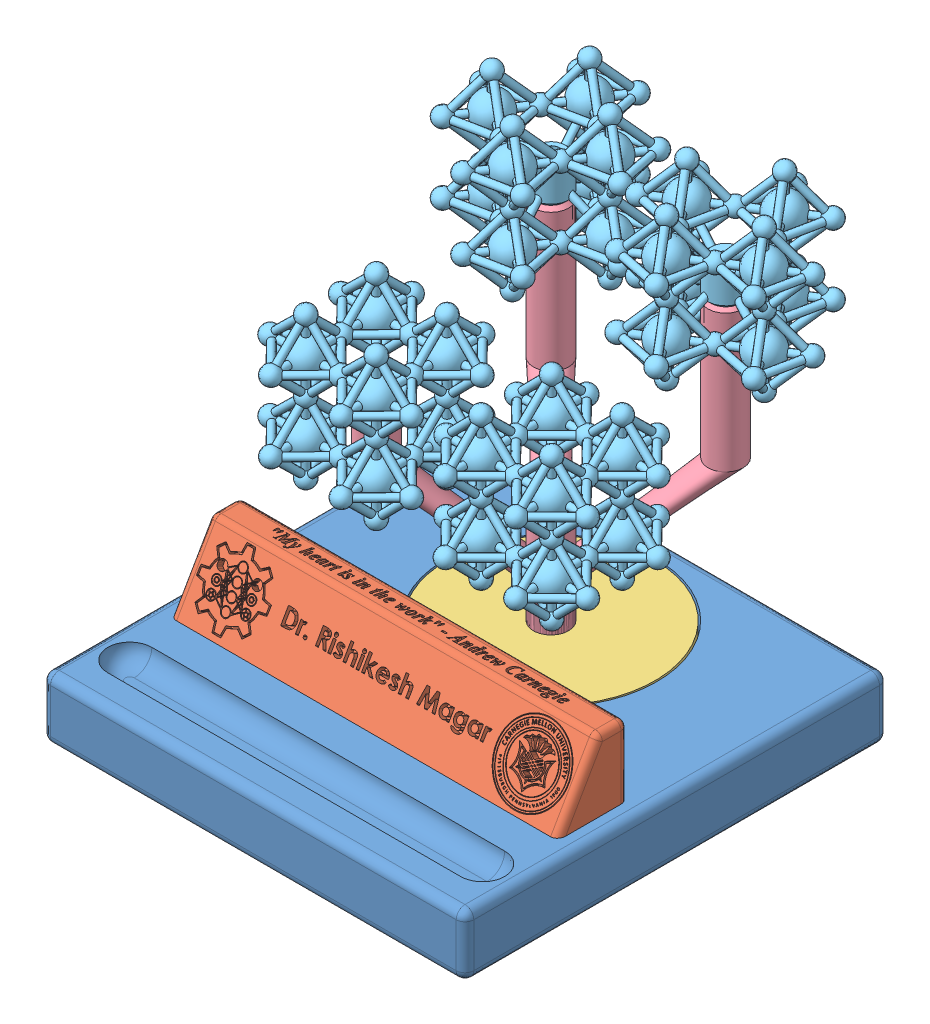
SolidWorks assembly PenHolderV1, configuration Default. Lengths in mm.
Overall size (152.4 158.62 177.96).
8 component instances, 5 part files, 5 mates.
Components (placement in the parent):
- Base-1: Base [9246K573] at origin size (152.4 22.23 152.4)
- NamePlate-1: NamePlate [Default] at (0 11.1125 23.8125) size (139.7 25.4 25.4)
- Mount-1: Mount [Default] at (0 -1.5875 -30.9563) size (74.93 12.7 74.93)
- PerovskiteMount-1: PerovskiteMount [Default] at (0 11.1125 -30.9563) size (75.84 101.6 75.84)
- PerovskiteStructure-2: PerovskiteStructure [Default] at (-18.7309 93.9375 -12.2254) x (-1 0 0) z (0 0 1) size (57.15 57.15 57.15)
- PerovskiteStructure-6: PerovskiteStructure [Default] at (-49.0091 131.7625 -58.7013) x (0.837169 0 0.546944) z (0.546944 0 -0.837169) size (57.15 57.15 57.15)
- PerovskiteStructure-7: PerovskiteStructure [Default] at (18.7309 93.9375 12.9181) x (1 0 0) z (0 0 -1) size (57.15 57.15 57.15)
- PerovskiteStructure-8: PerovskiteStructure [Default] at (49.0091 106.1059 -58.7013) x (-0.837169 0 0.546944) z (-0.546944 0 -0.837169) size (57.15 57.15 57.15)
Mates (geometry in assembly coordinates):
- Coincident3: coincident anti-aligned: plane of Base-1 through (-76.2 11.1125 76.2) normal (0 1 0); plane of NamePlate-1 through (0 11.1125 23.8125) normal (0 -1 0)
- Distance11: distance = 12.7 mm: line of NamePlate-1 through (-67.31 11.1125 36.5125) axis (1 0 0); line of Base-1 through (63.5 11.1125 49.2125) axis (-1 0 0)
- Concentric2: concentric anti-aligned: circle of Base-1; circle of Mount-1
- Coincident4: coincident anti-aligned: point of Mount-1; moEndPointRef_w of PerovskiteMount-1
- Coincident8: coincident anti-aligned: plane of PerovskiteMount-1 through (-31.4309 112.7125 -62.3871) normal (0 1 0); plane of PerovskiteStructure-6 through (-31.4309 112.7125 -62.3871) normal (0 -1 0)
